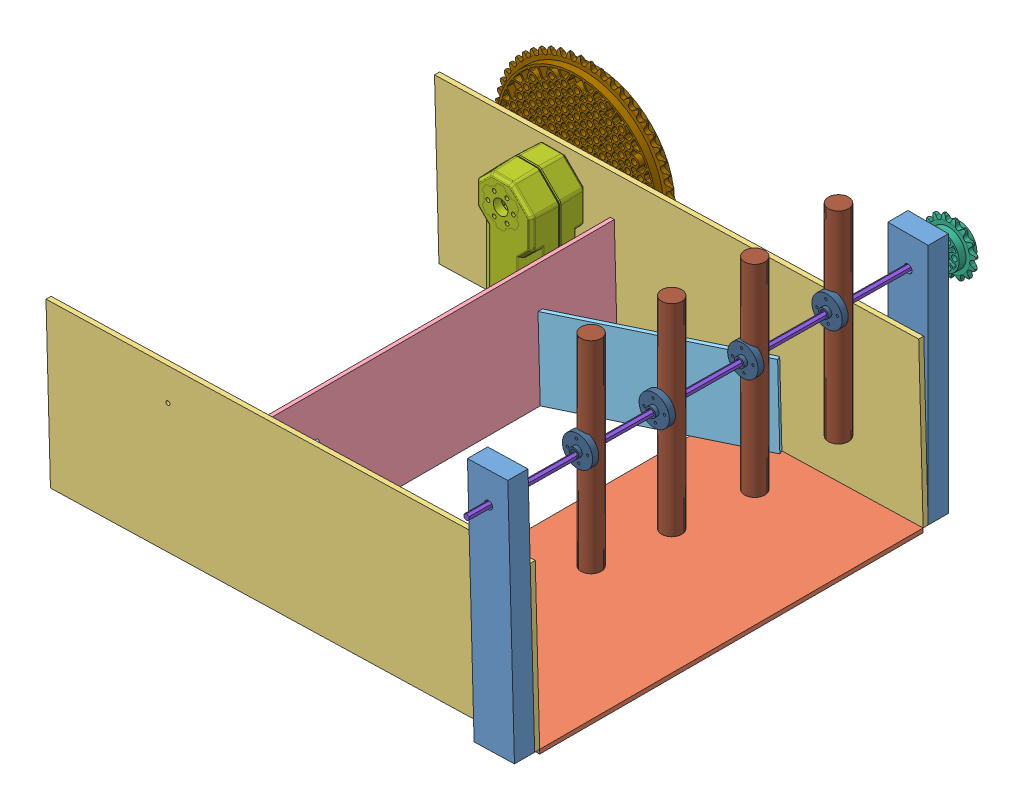
SolidWorks assembly FINALIntake, configuration Default. Lengths in mm.
Overall size (313.05 203.09 307.6).
20 component instances, 11 part files, 27 mates.
Components (placement in the parent):
- entraceBoiz-1: entraceBoiz [Default] at (-33.4348 37.864 140.8285) size (25.4 152.4 12.7)
- entraceBoiz-2: entraceBoiz [Default] at (-33.4252 37.1675 401.1785) x (0.999624 0.027421 0) z (0 0 1) size (25.4 152.4 12.7)
- bottomSlab-1: bottomSlab [Default] at (-7.9651 35.325 385.3035) x (0 0 -1) z (0.999624 0.027421 0) size (241.3 2.54 127)
- bigPolySides-1: bigPolySides [Default] at (-315.5061 131.0679 385.3035) x (0.999624 0.027421 0) z (0.027421 -0.999624 0) size (304.8 3.17 101.6)
- bigPolySides-2: bigPolySides [Default] at (-315.5061 131.0679 140.8285) x (0.999624 0.027421 0) z (0.027421 -0.999624 0) size (304.8 3.17 101.6)
- stopperBoi-1: stopperBoi [Default] at (-202.8379 32.5203 408.1635) x (0 0 -1) z (0.027421 -0.999624 0) size (243.84 2.54 76.2)
- funnel-1: funnel [Default] at (-96.9164 35.4259 144.0035) x (-0.027421 0.999624 0) z (0.913619 0.025062 -0.405798) size (50.8 2.54 114.3)
- funnel-2: funnel [Default] at (-98.1808 35.3912 383.0373) x (-0.027421 0.999624 0) z (0.891856 0.024465 0.451657) size (50.8 2.54 114.3)
- PART_Sprocket15Tooth-1: PART_Sprocket15Tooth [Default] at (-19.5878 171.2468 115.0943) x (0.999814 0.013943 0.013351) z (-0.013318 -0.002434 0.999908) size (33.59 33.42 15)
- PART_MotorCoreHex_Shell-1: PART_MotorCoreHex_Shell [Default] at (-239.4155 114.1875 160.2535) x (0 1 0) z (0 0 -1) size (100 42.79 34.54)
- hexShaft12in-1: hexShaft12in [Default] at (-19.3078 172.2358 110.152) x (-0.013889 0.999901 0.002249) z (0.999815 0.013857 0.01335) size (3.67 304.8 3.18)
- PART_Sprocket54Tooth-1: PART_Sprocket54Tooth [Default] at (-238.498 112.9014 125.9042) size (112.84 112.69 15)
- motorHub-1: motorHub [Default] at (-21.8385 172.0247 239.8648) x (0 1 0) z (1 0 0) size (19.05 6.1 19.05)
- motorHub-2: motorHub [Default] at (-21.7027 172.3795 186.9767) x (1 0 0) z (0 -1 0) size (19.05 6.1 19.05)
- motorHub-3: motorHub [Default] at (-22.6424 171.9626 294.81) x (1 0 0) z (0 -1 0) size (19.05 6.1 19.05)
- motorHub-4: motorHub [Default] at (-24.0392 172.5447 341.6512) x (1 0 0) z (0 -1 0) size (19.05 6.1 19.05)
- surgTub-1: surgTub [Default] at (-23.5513 99.1704 181.7557) size (12.7 127 12.7)
- surgTub-2: surgTub [Default] at (-21.7297 98.2488 236.2748) size (12.7 127 12.7)
- surgTub-3: surgTub [Default] at (-21.9126 102.7709 288.3248) size (12.7 127 12.7)
- surgTub-4: surgTub [Default] at (-24.2573 105.5969 336.726) size (12.7 127 12.7)
Mates (geometry in assembly coordinates):
- Coincident1: coincident anti-aligned: line of bottomSlab-1 through (-8.0348 37.864 144.0035) axis (-0.999624 -0.027421 0); line of bigPolySides-2 through (-312.7202 29.5061 144.0035) axis (0.999624 0.027421 0)
- Coincident2: coincident aligned: line of bottomSlab-1 through (-134.987 34.3816 385.3035) axis (0.999624 0.027421 0); line of bigPolySides-1 through (-312.7202 29.5061 385.3035) axis (0.999624 0.027421 0)
- Coincident3: coincident anti-aligned: plane of entraceBoiz-1 through (-33.4348 190.264 140.8285) normal (0 0 1); plane of bigPolySides-2 through (-315.5061 131.0679 140.8285) normal (0 0 -1)
- Coincident4: coincident anti-aligned: plane of entraceBoiz-2 through (-37.6042 189.5102 388.4785) normal (0 0 -1); plane of bigPolySides-1 through (-315.5061 131.0679 388.4785) normal (0 0 1)
- Perpendicular1: perpendicular: plane of bottomSlab-1 through (-8.0348 37.864 385.3035) normal (-0.027421 0.999624 0); plane of bigPolySides-2 through (-315.5061 131.0679 144.0035) normal (0 0 1)
- Perpendicular2: perpendicular: plane of bottomSlab-1 through (-8.0348 37.864 385.3035) normal (-0.027421 0.999624 0); plane of bigPolySides-1 through (-315.5061 131.0679 385.3035) normal (0 0 -1)
- Coincident6: coincident aligned: line of bottomSlab-1 through (-8.0348 37.864 385.3035) axis (0 0 -1); line of bigPolySides-2 through (-8.0348 37.864 144.0035) axis (0 0 -1)
- Coincident7: coincident aligned: line of bottomSlab-1 through (-8.0348 37.864 385.3035) axis (0 0 -1); line of bigPolySides-1 through (-8.0348 37.864 388.4785) axis (0 0 -1)
- Coincident8: coincident anti-aligned: line of entraceBoiz-2 through (-12.2137 190.2067 388.4785) axis (0.027421 -0.999624 0); line of bigPolySides-1 through (-8.0348 37.864 388.4785) axis (-0.027421 0.999624 0)
- Coincident9: coincident aligned: line of entraceBoiz-2 through (-8.0348 37.864 401.1785) axis (0 0 -1); line of bigPolySides-1 through (-8.0348 37.864 388.4785) axis (0 0 -1)
- Coincident10: coincident aligned: line of entraceBoiz-1 through (-8.0348 37.864 140.8285) axis (0 0 -1); line of bigPolySides-2 through (-8.0348 37.864 144.0035) axis (0 0 -1)
- Coincident11: coincident anti-aligned: plane of bigPolySides-1 through (-315.5061 131.0679 385.3035) normal (0 0 -1); plane of stopperBoi-1 through (-202.8379 32.5203 385.3035) normal (0 0 1)
- Coincident12: coincident aligned: line of bigPolySides-1 through (-312.7202 29.5061 385.3035) axis (0.999624 0.027421 0); line of stopperBoi-1 through (-202.8379 32.5203 385.3035) axis (0.999624 0.027421 0)
- Perpendicular3: perpendicular: plane of stopperBoi-1 through (-200.2989 32.59 408.1635) normal (0.999624 0.027421 0); plane of funnel-1 through (-97.279 86.235 146.3249) normal (-0.027421 0.999624 0)
- Coincident14: coincident: plane of bigPolySides-2 through (-315.5061 131.0679 144.0035) normal (0 0 1); line of funnel-1 through (-96.9164 35.4259 144.0035) axis (-0.027421 0.999624 0)
- Coincident16: coincident anti-aligned: plane of bottomSlab-1 through (-8.0348 37.864 385.3035) normal (-0.027421 0.999624 0); plane of funnel-1 through (-95.886 35.4541 146.3249) normal (0.027421 -0.999624 0)
- Perpendicular4: perpendicular: plane of stopperBoi-1 through (-200.2989 32.59 408.1635) normal (0.999624 0.027421 0); plane of funnel-2 through (-100.7205 86.1406 385.3035) normal (-0.027421 0.999624 0)
- Coincident18: coincident: plane of bigPolySides-1 through (-315.5061 131.0679 385.3035) normal (0 0 -1); line of funnel-2 through (-99.3276 35.3597 385.3035) axis (-0.027421 0.999624 0)
- Coincident19: coincident anti-aligned: plane of bottomSlab-1 through (-8.0348 37.864 385.3035) normal (-0.027421 0.999624 0); plane of funnel-2 through (-99.3276 35.3597 385.3035) normal (0.027421 -0.999624 0)
- Coincident20: coincident anti-aligned: plane of bigPolySides-2 through (-315.5061 131.0679 144.0035) normal (0 0 1); plane of PART_MotorCoreHex_Shell-1 through (-238.0114 104.4408 144.0035) normal (0 0 -1)
- Lock1: lock: unknown of entraceBoiz-1; unknown of hexShaft12in-1
- Coincident23: coincident anti-aligned: plane of PART_Sprocket15Tooth-1 through (-19.6096 174.1366 113.7059) normal (0.512009 -0.858967 0.004729); plane of hexShaft12in-1 through (-24.5265 172.864 414.9119) normal (-0.512009 0.858967 -0.004729)
- Coincident24: coincident anti-aligned: plane of PART_Sprocket15Tooth-1 through (-22.089 172.6585 113.6693) normal (0.999814 0.013943 0.013351); plane of hexShaft12in-1 through (-26.1009 171.9254 414.8887) normal (-0.999814 -0.013943 -0.013351)
- Lock2: lock: unknown of hexShaft12in-1; unknown of motorHub-2
- Lock3: lock: unknown of hexShaft12in-1; unknown of motorHub-1
- Lock4: lock: unknown of hexShaft12in-1; unknown of motorHub-3
- Lock5: lock: unknown of hexShaft12in-1; unknown of motorHub-4
